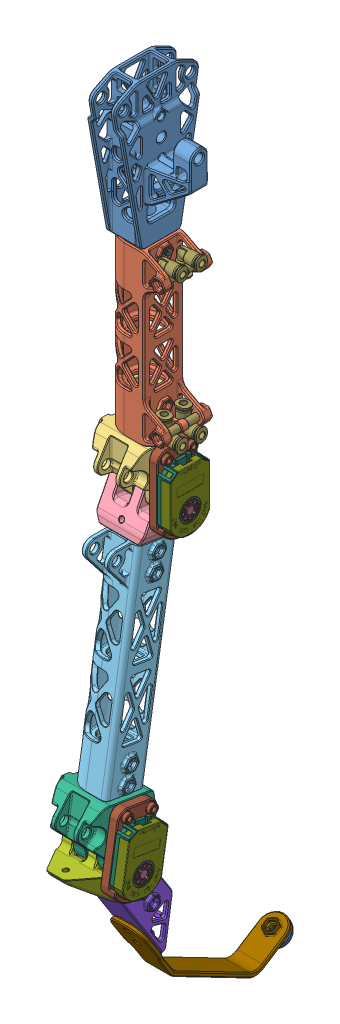
SolidWorks assembly AARL_Puppy_18_01_04_004, configuration Default. Lengths in mm.
Overall size (59.35 614.9 171.35).
42 component instances, 24 part files, 68 mates.
Components (placement in the parent):
- AARL_QR_FR_LE_PA_FR_028-2: AARL_QR_FR_LE_PA_FR_028 [Default] at (43.9453 155.049 100.762) size (52.49 127.48 60.54)
- AARL_QR_FR_LE_PL_BL_021-2: AARL_QR_FR_LE_PL_BL_021 [Default] at (43.9453 -3.9396 100.762) size (46.38 120.65 34.92)
- AARL_Puppy_18_01_04_037-1: AARL_Puppy_18_01_04_037 [Default] at (44.2247 -15.0521 100.762) x (0 0 1) z (1 0 0) size (54.18 69.85 37.51)
- AARL_QR_FR_LE_PL_BL_020-1: AARL_QR_FR_LE_PL_BL_020 [Default] at (44.1231 -40.4521 100.762) x (1 0 0) z (0 0.158913 0.987293) size (34.93 59.22 41.48)
- AARL_QR_FR_LE_PL_BL_024-1: AARL_QR_FR_LE_PL_BL_024 [Default] at (44.1231 -212.858 128.5122) x (1 0 0) z (0 0.158913 0.987293) size (30.96 149.23 44.46)
- AARL_Puppy_18_01_04_040-2: AARL_Puppy_18_01_04_040 [Default] at (95.2025 -223.8293 130.2781) x (0 -0.158913 -0.987293) z (-1 0 0) size (54.18 69.85 37.51)
- AARL_QR_FR_LE_PL_BL_013-1: AARL_QR_FR_LE_PL_BL_013 [Default] at (44.4025 -248.9066 134.3145) x (-1 0 0) z (0 0.539554 -0.841951) size (34.93 68.68 39.69)
- AARL_QR_FR_LE_PL_BL_014-1: AARL_QR_FR_LE_PL_BL_014 [Default] at (44.4025 -295.8585 104.2259) x (1 0 0) z (0 -0.539554 0.841951) size (27.78 53.98 25.4)
- AARL_QR_FR_LE_PL_BL_015-1: AARL_QR_FR_LE_PL_BL_015 [Default] at (44.4025 -304.904 115.3987) x (0 0.539554 -0.841951) z (1 0 0) size (70.12 107.32 25.4)
- AARL_QR_FR_LE_PL_BL_016-1: AARL_QR_FR_LE_PL_BL_016 [Default] at (44.4025 -363.4207 7.8107) x (0.981016 -0.104633 0.163276) z (0 0.841951 0.539554) size (18.99 18.99 9.09)
- AARL_Puppy_18_01_04_043-1: AARL_Puppy_18_01_04_043 [Default] at (61.7888 -40.4521 100.762) x (0 0 1) z (1 0 0) size (29.26 55.03 14.11)
- AARL_Puppy_18_01_04_043-2: AARL_Puppy_18_01_04_043 [Default] at (61.9666 -248.9066 134.3145) x (0 0.158913 0.987293) z (1 0 0) size (29.26 55.03 14.11)
- AARL_QR_PN_FT_002-QSML-4-4: AARL_QR_PN_FT_002-QSML-4 [Standard] at (65.4328 3.2604 107.6205) x (1 0 0) z (0 1 0) size (18.4 8 18.4)
- AARL_QR_PN_FT_002-QSML-4-6: AARL_QR_PN_FT_002-QSML-4 [Standard] at (65.4328 3.2604 93.9035) x (1 0 0) z (0 1 0) size (18.4 8 18.4)
- AARL_QR_PN_FT_002-QSML-4-7: AARL_QR_PN_FT_002-QSML-4 [Standard] at (65.4328 109.5104 93.9035) x (0 -1 0) z (1 0 0) size (18.4 8 18.4)
- AARL_QR_PN_FT_002-QSML-4-8: AARL_QR_PN_FT_002-QSML-4 [Standard] at (65.4328 109.5104 107.6205) x (0 -1 0) z (1 0 0) size (18.4 8 18.4)
- AARL_QR_HW_ST_002-8632T132_D_PROFILE_SHAFT_SHORT-3: AARL_QR_HW_ST_002-8632T132_D_PROFILE_SHAFT_SHORT [8632T132] at (51.9763 -40.4521 100.762) x (0 -0.999942 0.010793) z (-1 0 0) size (6.35 6.35 50.8)
- AARL_QR_HW_ST_002-8632T132_D_PROFILE_SHAFT_SHORT-4: AARL_QR_HW_ST_002-8632T132_D_PROFILE_SHAFT_SHORT [8632T132] at (52.1541 -248.9066 134.3145) x (0 0.841951 0.539554) z (-1 0 0) size (6.35 6.35 50.8)
- AARL_QR_HW_BE_004-6377K310_ULTRA-LOW-FRICTION DRY-RUNNING SLEEVE BEARING-1: AARL_QR_HW_BE_004-6377K310_ULTRA-LOW-FRICTION DRY-RUNNING SLEEVE BEARING [6377K31] at (58.6138 -40.4521 100.762) x (0 0.211282 -0.977425) z (1 0 0) size (9.55 9.55 6.35)
- AARL_QR_HW_BE_004-6377K310_ULTRA-LOW-FRICTION DRY-RUNNING SLEEVE BEARING-2: AARL_QR_HW_BE_004-6377K310_ULTRA-LOW-FRICTION DRY-RUNNING SLEEVE BEARING [6377K31] at (37.8747 -40.4521 100.762) x (0 0 -1) z (1 0 0) size (9.55 9.55 6.35)
- AARL_QR_EL_EN2-amt102-0048-i6350-s-1: AARL_QR_EL_EN2-amt102-0048-i6350-s [Default] at (71.9963 -40.4527 100.761) x (0 -0.000059 1) z (1 0 0) size (36.33 46.23 9.15)
  - AARL_QR_EL_EN2_001-CUI_DEVICES_amt-102-base-rev-k-1: AARL_QR_EL_EN2_001-CUI_DEVICES_amt-102-base-rev-k [Default] x (-1 0 0) z (0 0 -1) size (28.83 43.41 9.03)
  - AARL_QR_EL_EN2_002-CUI_DEVICES_amt-102-top-cover-rev-h-1: AARL_QR_EL_EN2_002-CUI_DEVICES_amt-102-top-cover-rev-h [Default] at (0 0 5.23) x (-1 0 0) z (0 0 -1) size (28.6 43.26 6.55)
  - AARL_QR_EL_EN2_003-CUI_DEVICES_amt-sleeve-rev-d(d)-1: AARL_QR_EL_EN2_003-CUI_DEVICES_amt-sleeve-rev-d(d) [Default] at (0 0 -2.42) x (0.999996 0.002864 0) z (0 0 1) size (10.79 10.79 7.8)
  - AARL_QR_EL_EN2_004-CUI_DEVICES_amt-hub-top-rev-d1-1: AARL_QR_EL_EN2_004-CUI_DEVICES_amt-hub-top-rev-d1 [Default] at (0 0 2.13) x (0.999996 0.002864 0) z (0 0 1) size (14 14 5.67)
  - AARL_QR_EL_EN2_005-CUI_DEVICES_amt-hub-bottom-rev-b-1: AARL_QR_EL_EN2_005-CUI_DEVICES_amt-hub-bottom-rev-b [Default] at (0 0 2.43) x (0.999998 -0.001942 0) z (0 0 1) size (17.3 17.3 3.2)
  - AARL_QR_EL_EN2_006-CUI_DEVICES_amt10x-shaft-adaptor-rev-e-1: AARL_QR_EL_EN2_006-CUI_DEVICES_amt10x-shaft-adaptor-rev-e [Default] at (0 0 0.03) x (0.999996 0.002864 0) z (0 0 1) size (11.8 11.8 7.8)
  - AARL_QR_EL_EN2_007-CUI_DEVICES_receiver-board-1: AARL_QR_EL_EN2_007-CUI_DEVICES_receiver-board [Default] at (72.2834 -20.351 3.03) x (-1 0 0) z (0 0 -1) size (26.5 26.62 0.41)
  - AARL_QR_EL_EN2_008-CUI_DEVICES_rotor-board-rev f-1: AARL_QR_EL_EN2_008-CUI_DEVICES_rotor-board-rev f [Default] at (0 0 2.13) x (0.807874 -0.589355 0) z (0 0 1) size (26 26 0.3)
  - AARL_QR_EL_EN2_009-CUI_DEVICES_transmitter-board amt10(amt-102)-1: AARL_QR_EL_EN2_009-CUI_DEVICES_transmitter-board amt10(amt-102) [Default] at (19.1596 -17.1102 1.22) x (-1 0 0) z (0 0 -1) size (26.63 38.43 4.41)
- AARL_QR_EL_EN2-amt102-0048-i6350-s-2: AARL_QR_EL_EN2-amt102-0048-i6350-s [Default] at (72.1741 -248.9073 134.3137) x (0 0.158855 0.987302) z (1 0 0) size (36.33 46.23 9.15)
  - AARL_QR_EL_EN2_001-CUI_DEVICES_amt-102-base-rev-k-1: AARL_QR_EL_EN2_001-CUI_DEVICES_amt-102-base-rev-k [Default] x (-1 0 0) z (0 0 -1) size (28.83 43.41 9.03)
  - AARL_QR_EL_EN2_002-CUI_DEVICES_amt-102-top-cover-rev-h-1: AARL_QR_EL_EN2_002-CUI_DEVICES_amt-102-top-cover-rev-h [Default] at (0 0 5.23) x (-1 0 0) z (0 0 -1) size (28.6 43.26 6.55)
  - AARL_QR_EL_EN2_003-CUI_DEVICES_amt-sleeve-rev-d(d)-1: AARL_QR_EL_EN2_003-CUI_DEVICES_amt-sleeve-rev-d(d) [Default] at (0 0 -2.42) x (0.999996 0.002864 0) z (0 0 1) size (10.79 10.79 7.8)
  - AARL_QR_EL_EN2_004-CUI_DEVICES_amt-hub-top-rev-d1-1: AARL_QR_EL_EN2_004-CUI_DEVICES_amt-hub-top-rev-d1 [Default] at (0 0 2.13) x (0.999996 0.002864 0) z (0 0 1) size (14 14 5.67)
  - AARL_QR_EL_EN2_005-CUI_DEVICES_amt-hub-bottom-rev-b-1: AARL_QR_EL_EN2_005-CUI_DEVICES_amt-hub-bottom-rev-b [Default] at (0 0 2.43) x (0.999998 -0.001942 0) z (0 0 1) size (17.3 17.3 3.2)
  - AARL_QR_EL_EN2_006-CUI_DEVICES_amt10x-shaft-adaptor-rev-e-1: AARL_QR_EL_EN2_006-CUI_DEVICES_amt10x-shaft-adaptor-rev-e [Default] at (0 0 0.03) x (0.999996 0.002864 0) z (0 0 1) size (11.8 11.8 7.8)
  - AARL_QR_EL_EN2_007-CUI_DEVICES_receiver-board-1: AARL_QR_EL_EN2_007-CUI_DEVICES_receiver-board [Default] at (72.2834 -20.351 3.03) x (-1 0 0) z (0 0 -1) size (26.5 26.62 0.41)
  - AARL_QR_EL_EN2_008-CUI_DEVICES_rotor-board-rev f-1: AARL_QR_EL_EN2_008-CUI_DEVICES_rotor-board-rev f [Default] at (0 0 2.13) x (0.807874 -0.589355 0) z (0 0 1) size (26 26 0.3)
  - AARL_QR_EL_EN2_009-CUI_DEVICES_transmitter-board amt10(amt-102)-1: AARL_QR_EL_EN2_009-CUI_DEVICES_transmitter-board amt10(amt-102) [Default] at (19.1596 -17.1102 1.22) x (-1 0 0) z (0 0 -1) size (26.63 38.43 4.41)
- AARL_QR_HW_CS_029-1: AARL_QR_HW_CS_029 [Default] at (26.813 110.3604 100.762) x (0 -0.235908 -0.971775) z (0 -0.971775 0.235908) size (4.65 34.79 4.65)
- AARL_QR_HW_CS_029-2: AARL_QR_HW_CS_029 [Default] at (26.813 97.6604 100.762) x (0 -0.235908 -0.971775) z (0 -0.971775 0.235908) size (4.65 34.79 4.65)
Mates (geometry in assembly coordinates):
- Concentric11: concentric aligned: cylinder of AARL_Puppy_18_01_04_040-2 through (75.6166 -248.9066 134.3145) axis (-1 0 0) radius 4.826; cylinder of AARL_QR_FR_LE_PL_BL_013-1 through (61.865 -248.9066 134.3145) axis (-1 0 0) radius 3.2385
- Coincident3: coincident anti-aligned: plane of AARL_Puppy_18_01_04_040-2; plane of AARL_QR_FR_LE_PL_BL_013-1 through (44.4025 -248.9066 134.3145) normal (-1 0 0)
- LimitAngle3: limit planar angle = 0.729498 rad anti-aligned: plane of AARL_QR_FR_LE_PL_BL_013-1 through (-20.4418 -252.7442 143.3393) normal (0 0.99672 -0.080932); plane of AARL_Puppy_18_01_04_040-2 through (100.8116 -231.1789 156.3642) normal (0 -0.689123 0.724644)
- Parallel4: parallel anti-aligned: plane of AARL_Puppy_18_01_04_040-2 through (100.8116 -210.5714 142.7184) normal (0 0.987293 -0.158913); plane of AARL_QR_FR_LE_PL_BL_013-1 through (44.4025 -294.5219 105.0824) normal (0 -0.841951 -0.539554)
- Parallel7: parallel anti-aligned: plane of AARL_QR_FR_LE_PL_BL_013-1 through (61.865 -248.7202 131.0814) normal (0 -0.539554 0.841951); plane of AARL_QR_HW_ST_002-8632T132_D_PROFILE_SHAFT_SHORT-4 through (26.7541 -248.7596 131.1429) normal (0 0.539554 -0.841951)
- Concentric25: concentric aligned: cylinder of AARL_Puppy_18_01_04_037-1 through (75.4388 -40.4521 100.762) axis (-1 0 0) radius 4.826; cylinder of AARL_QR_HW_BE_004-6377K310_ULTRA-LOW-FRICTION DRY-RUNNING SLEEVE BEARING-1 through (61.7888 -40.4521 100.762) axis (-1 0 0) radius 4.7752
- Coincident13: coincident anti-aligned: plane of AARL_Puppy_18_01_04_037-1 through (55.4388 -40.4521 100.762) normal (1 0 0); plane of AARL_QR_HW_BE_004-6377K310_ULTRA-LOW-FRICTION DRY-RUNNING SLEEVE BEARING-1 through (55.4388 -40.4521 100.762) normal (-1 0 0)
- Concentric26: concentric anti-aligned: cylinder of AARL_Puppy_18_01_04_037-1 through (21.0497 -40.4521 100.762) axis (1 0 0) radius 4.826; cylinder of AARL_QR_HW_BE_004-6377K310_ULTRA-LOW-FRICTION DRY-RUNNING SLEEVE BEARING-2 through (41.0497 -40.4521 100.762) axis (-1 0 0) radius 4.7752
- Coincident14: coincident anti-aligned: plane of AARL_Puppy_18_01_04_037-1 through (41.0497 -40.4521 100.762) normal (-1 0 0); plane of AARL_QR_HW_BE_004-6377K310_ULTRA-LOW-FRICTION DRY-RUNNING SLEEVE BEARING-2 through (41.0497 -40.4521 100.762) normal (1 0 0)
- Concentric27: concentric aligned: cylinder of AARL_Puppy_18_01_04_037-1 through (26.6606 -8.7021 91.872) axis (1 0 0) radius 1.5875; cylinder of AARL_Puppy_18_01_04_043-1 through (61.7888 -8.7021 91.872) axis (1 0 0) radius 1.5875
- Concentric28: concentric aligned: cylinder of AARL_Puppy_18_01_04_037-1 through (26.6606 -8.7021 109.652) axis (1 0 0) radius 1.5875; cylinder of AARL_Puppy_18_01_04_043-1 through (61.7888 -8.7021 109.652) axis (1 0 0) radius 1.5875
- Coincident15: coincident anti-aligned: plane of AARL_Puppy_18_01_04_037-1 through (61.7888 -40.4521 100.762) normal (1 0 0); plane of AARL_Puppy_18_01_04_043-1 through (61.7888 -40.2997 100.762) normal (-1 0 0)
- Concentric29: concentric aligned: cylinder of AARL_Puppy_18_01_04_040-2 through (26.8384 -218.9728 120.492) axis (1 0 0) radius 1.5875; cylinder of AARL_Puppy_18_01_04_043-2 through (61.9666 -218.9728 120.492) axis (1 0 0) radius 1.5875
- Concentric30: concentric aligned: cylinder of AARL_Puppy_18_01_04_040-2 through (26.8384 -216.1473 138.046) axis (1 0 0) radius 1.5875; cylinder of AARL_Puppy_18_01_04_043-2 through (61.9666 -216.1473 138.046) axis (1 0 0) radius 1.5875
- Coincident16: coincident anti-aligned: plane of AARL_Puppy_18_01_04_040-2 through (61.9666 -248.9066 134.3145) normal (1 0 0); plane of AARL_Puppy_18_01_04_043-2 through (61.9666 -248.7561 134.2903) normal (-1 0 0)
- Concentric31: concentric anti-aligned: cylinder of AARL_QR_EL_EN2-amt102-0048-i6350-s-1/AARL_QR_EL_EN2_001-CUI_DEVICES_amt-102-base-rev-k-1 through (68.2263 -24.7041 90.2845) axis (1 0 0) radius 1.9812; cylinder of AARL_Puppy_18_01_04_043-1 through (70.7663 -24.7041 90.2845) axis (-1 0 0) radius 1.8542
- Concentric32: concentric anti-aligned: cylinder of AARL_QR_EL_EN2-amt102-0048-i6350-s-1/AARL_QR_EL_EN2_001-CUI_DEVICES_amt-102-base-rev-k-1 through (68.2263 -49.4335 109.7407) axis (1 0 0) radius 1.9812; cylinder of AARL_Puppy_18_01_04_043-1 through (70.7663 -49.4337 109.7409) axis (-1 0 0) radius 1.8542
- Coincident17: coincident anti-aligned: plane of AARL_QR_EL_EN2-amt102-0048-i6350-s-1/AARL_QR_EL_EN2_001-CUI_DEVICES_amt-102-base-rev-k-1 through (68.2263 -30.0327 100.7616) normal (-1 0 0); plane of AARL_Puppy_18_01_04_043-1 through (68.2263 -40.2997 100.762) normal (1 0 0)
- Coincident18: coincident aligned: plane of AARL_QR_HW_ST_002-8632T132_D_PROFILE_SHAFT_SHORT-3 through (77.3763 -40.4521 100.762) normal (1 0 0); plane of AARL_QR_EL_EN2-amt102-0048-i6350-s-1/AARL_QR_EL_EN2_003-CUI_DEVICES_amt-sleeve-rev-d(d)-1 through (77.3763 -40.4527 100.761) normal (1 0 0)
- Concentric33: concentric anti-aligned: cylinder of AARL_QR_HW_ST_002-8632T132_D_PROFILE_SHAFT_SHORT-3 through (26.5763 -40.4521 100.762) axis (1 0 0) radius 3.175; cylinder of AARL_QR_HW_BE_004-6377K310_ULTRA-LOW-FRICTION DRY-RUNNING SLEEVE BEARING-2 through (41.0497 -40.4521 100.762) axis (-1 0 0) radius 3.2258
- Concentric34: concentric anti-aligned: cylinder of AARL_QR_EL_EN2-amt102-0048-i6350-s-2/AARL_QR_EL_EN2_001-CUI_DEVICES_amt-102-base-rev-k-1 through (68.4041 -235.0237 121.4676) axis (1 0 0) radius 1.9812; cylinder of AARL_Puppy_18_01_04_043-2 through (70.9441 -235.0237 121.4676) axis (-1 0 0) radius 1.8542
- Concentric35: concentric anti-aligned: cylinder of AARL_QR_EL_EN2-amt102-0048-i6350-s-2/AARL_QR_EL_EN2_001-CUI_DEVICES_amt-102-base-rev-k-1 through (68.4041 -256.347 144.6064) axis (1 0 0) radius 1.9812; cylinder of AARL_Puppy_18_01_04_043-2 through (70.9441 -256.3472 144.6066) axis (-1 0 0) radius 1.8542
- Coincident19: coincident anti-aligned: plane of AARL_QR_EL_EN2-amt102-0048-i6350-s-2/AARL_QR_EL_EN2_001-CUI_DEVICES_amt-102-base-rev-k-1 through (68.4041 -238.6196 132.6584) normal (-1 0 0); plane of AARL_Puppy_18_01_04_043-2 through (68.4041 -248.7561 134.2903) normal (1 0 0)
- Coincident20: coincident aligned: plane of AARL_QR_HW_ST_002-8632T132_D_PROFILE_SHAFT_SHORT-4 through (77.5541 -248.9066 134.3145) normal (1 0 0); plane of AARL_QR_EL_EN2-amt102-0048-i6350-s-2/AARL_QR_EL_EN2_003-CUI_DEVICES_amt-sleeve-rev-d(d)-1 through (77.5541 -248.9073 134.3137) normal (1 0 0)
- Concentric36: concentric aligned: cylinder of AARL_Puppy_18_01_04_040-2 through (21.2275 -248.9066 134.3145) axis (1 0 0) radius 4.826; cylinder of AARL_QR_HW_ST_002-8632T132_D_PROFILE_SHAFT_SHORT-4 through (26.7541 -248.9066 134.3145) axis (1 0 0) radius 3.175
- Parallel9: parallel anti-aligned: plane of AARL_QR_FR_LE_PL_BL_013-1 through (61.865 -248.7202 131.0814) normal (0 -0.539554 0.841951); plane of AARL_QR_HW_ST_002-8632T132_D_PROFILE_SHAFT_SHORT-4 through (26.7541 -248.7596 131.1429) normal (0 0.539554 -0.841951)
- Concentric37: concentric aligned: cylinder of AARL_QR_FR_LE_PL_BL_013-1 through (53.9275 -278.4828 115.3609) axis (1 0 0) radius 1.5875; cylinder of AARL_QR_FR_LE_PL_BL_014-1 through (31.7025 -278.4828 115.3609) axis (1 0 0) radius 1.5875
- Concentric38: concentric aligned: cylinder of AARL_QR_FR_LE_PL_BL_013-1 through (53.9275 -289.1756 108.5086) axis (1 0 0) radius 1.5875; cylinder of AARL_QR_FR_LE_PL_BL_014-1 through (31.7025 -289.1756 108.5086) axis (1 0 0) radius 1.5875
- Coincident21: coincident anti-aligned: plane of AARL_QR_FR_LE_PL_BL_013-1 through (53.9275 -289.3827 97.0628) normal (1 0 0); plane of AARL_QR_FR_LE_PL_BL_014-1 through (53.9275 -278.2756 126.8067) normal (-1 0 0)
- Concentric41: concentric anti-aligned: cylinder of AARL_QR_FR_LE_PL_BL_014-1 through (44.4025 -295.6886 89.2495) axis (0 -0.539554 0.841951) radius 1.5875; cylinder of AARL_QR_FR_LE_PL_BL_015-1 through (44.4025 -311.1069 113.3091) axis (0 0.539554 -0.841951) radius 1.5875
- Concentric42: concentric anti-aligned: cylinder of AARL_QR_FR_LE_PL_BL_014-1 through (44.4025 -306.3814 82.3972) axis (0 -0.539554 0.841951) radius 1.5875; cylinder of AARL_QR_FR_LE_PL_BL_015-1 through (44.4025 -321.7997 106.4568) axis (0 0.539554 -0.841951) radius 1.5875
- Coincident23: coincident anti-aligned: plane of AARL_QR_FR_LE_PL_BL_014-1 through (57.1025 -301.3743 115.7752) normal (0 -0.539554 0.841951); plane of AARL_QR_FR_LE_PL_BL_015-1 through (53.9275 -304.0475 114.0621) normal (0 0.539554 -0.841951)
- Concentric43: concentric aligned: cylinder of AARL_QR_FR_LE_PL_BL_015-1 through (44.4025 -363.4207 7.8107) axis (0 0.841951 0.539554) radius 1.5875; cylinder of AARL_QR_FR_LE_PL_BL_016-1 through (44.4025 -363.4207 7.8107) axis (0 0.841951 0.539554) radius 1.5875
- Coincident24: coincident anti-aligned: plane of AARL_QR_FR_LE_PL_BL_015-1 through (53.9275 -377.7233 30.1293) normal (0 -0.841951 -0.539554); plane of AARL_QR_FR_LE_PL_BL_016-1 through (45.9599 -363.5868 8.0699) normal (0 0.841951 0.539554)
- Concentric47: concentric: cylinder of AARL_QR_FR_LE_PL_BL_019-2 through (29.65 -45.2146 100.762) axis (1 0 0) radius 1.5875; cylinder of AARL_Puppy_18_01_04_037-1 through (26.6606 -45.2146 100.762) axis (1 0 0) radius 1.5875
- Concentric48: concentric: cylinder of AARL_QR_FR_LE_PL_BL_019-2 through (29.65 -57.9146 100.762) axis (1 0 0) radius 1.5875; cylinder of AARL_Puppy_18_01_04_037-1 through (26.6606 -57.9146 100.762) axis (1 0 0) radius 1.5875
- Coincident26: coincident: plane of AARL_QR_FR_LE_PL_BL_019-2 through (55.0578 -38.8646 89.6495) normal (-1 0 0); plane of AARL_Puppy_18_01_04_037-1 through (55.0578 -38.8646 111.5951) normal (1 0 0)
- Concentric50: concentric anti-aligned: cylinder of AARL_QR_FR_LE_PL_BL_020-1 through (61.5856 -40.4521 100.762) axis (-1 0 0) radius 3.2385; cylinder of AARL_QR_HW_ST_002-8632T132_D_PROFILE_SHAFT_SHORT-3 through (26.5763 -40.4521 100.762) axis (1 0 0) radius 3.175
- Width4: width anti-aligned: plane of AARL_QR_FR_LE_PL_BL_020-1 through (34.3822 -38.0213 90.7336) normal (1 0 0); plane of AARL_QR_FR_LE_PL_BL_020-1 through (44.5422 -38.0213 90.7336) normal (-1 0 0); plane of AARL_Puppy_18_01_04_037-1 through (44.2247 -21.4021 121.5011) normal (1 0 0); plane of AARL_Puppy_18_01_04_037-1 through (34.6997 -40.4521 100.762) normal (-1 0 0)
- Parallel10: parallel: plane of AARL_QR_FR_LE_PL_BL_019-2 through (43.9453 56.3874 115.0495) normal (0 0 1); plane of AARL_QR_FR_LE_PL_BL_020-1
- Concentric51: concentric: cylinder of AARL_QR_FR_LE_PL_BL_019-2 through (70.9328 -51.5646 111.8745) axis (0 0 1) radius 1.5875; cylinder of AARL_QR_PN_FT_002-QSML-4-4 through (70.9328 -51.5646 103.6205) axis (0 0 -1) radius 1.6
- Width5: width: plane of AARL_QR_PN_FT_002-QSML-4-4 through (70.9328 8.7604 111.6205) normal (0 0 1); plane of AARL_QR_PN_FT_002-QSML-4-4 through (70.9328 8.7604 103.6205) normal (0 0 -1); plane of AARL_QR_FR_LE_PL_BL_019-2 through (43.9453 -3.9396 111.8745) normal (0 0 -1); plane of AARL_QR_FR_LE_PL_BL_019-2 through (43.9453 -3.9396 103.3665) normal (0 0 1)
- Concentric55: concentric aligned: cylinder of AARL_QR_FR_LE_PA_FR_028-2 through (31.2453 110.3604 100.762) axis (1 0 0) radius 1.5875; cylinder of AARL_QR_FR_LE_PL_BL_021-2 through (29.6578 110.3604 100.762) axis (1 0 0) radius 1.5875
- Concentric56: concentric aligned: cylinder of AARL_QR_FR_LE_PA_FR_028-2 through (31.2453 97.6604 100.762) axis (1 0 0) radius 1.5875; cylinder of AARL_QR_FR_LE_PL_BL_021-2 through (29.6578 97.6604 100.762) axis (1 0 0) radius 1.5875
- Coincident29: coincident anti-aligned: plane of AARL_QR_FR_LE_PA_FR_028-2 through (55.0578 59.8795 89.6495) normal (1 0 0); plane of AARL_QR_FR_LE_PL_BL_021-2 through (55.0578 116.7104 111.8745) normal (-1 0 0)
- Concentric58: concentric anti-aligned: cylinder of AARL_QR_FR_LE_PL_BL_021-2 through (70.9328 8.7604 111.8745) axis (0 0 1) radius 1.5875; cylinder of AARL_QR_PN_FT_002-QSML-4-4 through (70.9328 8.7604 103.6205) axis (0 0 -1) radius 1.6
- Width7: width anti-aligned: plane of AARL_QR_PN_FT_002-QSML-4-4 through (70.9328 8.7604 111.6205) normal (0 0 1); plane of AARL_QR_PN_FT_002-QSML-4-4 through (70.9328 8.7604 103.6205) normal (0 0 -1); plane of AARL_QR_FR_LE_PL_BL_021-2 through (43.9453 -3.9396 111.8745) normal (0 0 -1); plane of AARL_QR_FR_LE_PL_BL_021-2 through (43.9453 -3.9396 103.3665) normal (0 0 1)
- Concentric59: concentric aligned: cylinder of AARL_QR_FR_LE_PL_BL_021-2 through (70.9328 8.7604 89.6495) axis (0 0 -1) radius 1.5875; cylinder of AARL_QR_PN_FT_002-QSML-4-6 through (70.9328 8.7604 89.9035) axis (0 0 -1) radius 1.6
- Width8: width aligned: plane of AARL_QR_PN_FT_002-QSML-4-6 through (70.9328 8.7604 97.9035) normal (0 0 1); plane of AARL_QR_PN_FT_002-QSML-4-6 through (70.9328 8.7604 89.9035) normal (0 0 -1); plane of AARL_QR_FR_LE_PL_BL_021-2 through (43.9453 -3.9396 89.6495) normal (0 0 1); plane of AARL_QR_FR_LE_PL_BL_021-2 through (43.9453 -3.9396 98.1575) normal (0 0 -1)
- Concentric60: concentric aligned: cylinder of AARL_QR_FR_LE_PL_BL_021-2 through (70.9328 104.0104 89.6495) axis (0 0 -1) radius 1.5875; cylinder of AARL_QR_PN_FT_002-QSML-4-7 through (70.9328 104.0104 89.9035) axis (0 0 -1) radius 1.6
- Width9: width anti-aligned: plane of AARL_QR_PN_FT_002-QSML-4-7 through (70.9328 104.0104 97.9035) normal (0 0 1); plane of AARL_QR_PN_FT_002-QSML-4-7 through (70.9328 104.0104 89.9035) normal (0 0 -1); plane of AARL_QR_FR_LE_PL_BL_021-2 through (43.9453 -3.9396 98.1575) normal (0 0 -1); plane of AARL_QR_FR_LE_PL_BL_021-2 through (43.9453 -3.9396 89.6495) normal (0 0 1)
- Concentric61: concentric anti-aligned: cylinder of AARL_QR_FR_LE_PL_BL_021-2 through (70.9328 104.0104 111.8745) axis (0 0 1) radius 1.5875; cylinder of AARL_QR_PN_FT_002-QSML-4-8 through (70.9328 104.0104 103.6205) axis (0 0 -1) radius 1.6
- Width10: width anti-aligned: plane of AARL_QR_PN_FT_002-QSML-4-8 through (70.9328 104.0104 111.6205) normal (0 0 1); plane of AARL_QR_PN_FT_002-QSML-4-8 through (70.9328 104.0104 103.6205) normal (0 0 -1); plane of AARL_QR_FR_LE_PL_BL_021-2 through (43.9453 -3.9396 111.8745) normal (0 0 -1); plane of AARL_QR_FR_LE_PL_BL_021-2 through (43.9453 -3.9396 103.3665) normal (0 0 1)
- Concentric62: concentric anti-aligned: cylinder of AARL_QR_PN_FT_002-QSML-4-6 through (65.4328 16.7604 93.9035) axis (0 -1 0) radius 2; cylinder of AARL_QR_PN_FT_002-QSML-4-7 through (65.4328 96.0104 93.9035) axis (0 1 0) radius 2
- Concentric63: concentric anti-aligned: cylinder of AARL_QR_PN_FT_002-QSML-4-4 through (65.4328 16.7604 107.6205) axis (0 -1 0) radius 2; cylinder of AARL_QR_PN_FT_002-QSML-4-8 through (65.4328 96.0104 107.6205) axis (0 1 0) radius 2
- Concentric64: concentric aligned: cylinder of AARL_QR_FR_LE_PL_BL_021-2 through (29.6578 15.1104 100.762) axis (1 0 0) radius 1.5875; cylinder of AARL_Puppy_18_01_04_037-1 through (26.6606 15.1104 100.762) axis (1 0 0) radius 1.5875
- Concentric65: concentric aligned: cylinder of AARL_QR_FR_LE_PL_BL_021-2 through (29.6578 2.4104 100.762) axis (1 0 0) radius 1.5875; cylinder of AARL_Puppy_18_01_04_037-1 through (26.6606 2.4104 100.762) axis (1 0 0) radius 1.5875
- Coincident30: coincident anti-aligned: plane of AARL_QR_FR_LE_PL_BL_021-2 through (55.0578 21.4604 89.6495) normal (-1 0 0); plane of AARL_Puppy_18_01_04_037-1 through (55.0578 21.4604 111.5951) normal (1 0 0)
- Concentric72: concentric aligned: cylinder of AARL_QR_FR_LE_PL_BL_020-1 through (26.6606 -71.7986 105.8075) axis (1 0 0) radius 1.5875; cylinder of AARL_QR_FR_LE_PL_BL_024-1 through (29.8356 -71.7986 105.8075) axis (1 0 0) radius 1.5875
- Concentric73: concentric aligned: cylinder of AARL_QR_FR_LE_PL_BL_020-1 through (26.6606 -84.3372 107.8256) axis (1 0 0) radius 1.5875; cylinder of AARL_QR_FR_LE_PL_BL_024-1 through (29.8356 -84.3372 107.8256) axis (1 0 0) radius 1.5875
- Coincident33: coincident anti-aligned: plane of AARL_QR_FR_LE_PL_BL_020-1 through (55.2356 -88.8406 119.806) normal (1 0 0); plane of AARL_QR_FR_LE_PL_BL_024-1 through (55.2356 -63.7634 115.7696) normal (-1 0 0)
- Concentric74: concentric aligned: cylinder of AARL_QR_FR_LE_PL_BL_024-1 through (29.8356 -194.0501 125.4849) axis (1 0 0) radius 1.5875; cylinder of AARL_Puppy_18_01_04_040-2 through (26.8384 -194.0501 125.4849) axis (1 0 0) radius 1.5875
- Concentric75: concentric aligned: cylinder of AARL_QR_FR_LE_PL_BL_024-1 through (29.8356 -206.5887 127.5031) axis (1 0 0) radius 1.5875; cylinder of AARL_Puppy_18_01_04_040-2 through (26.8384 -206.5887 127.5031) axis (1 0 0) radius 1.5875
- Coincident34: coincident anti-aligned: plane of AARL_QR_FR_LE_PL_BL_024-1 through (55.2356 -189.5467 113.5045) normal (-1 0 0); plane of AARL_Puppy_18_01_04_040-2 through (55.2356 -189.5023 113.7803) normal (1 0 0)
- Concentric76: concentric anti-aligned: cylinder of AARL_QR_FR_LE_PL_BL_021-2 through (29.6578 110.3604 100.762) axis (1 0 0) radius 1.5875; cylinder of AARL_QR_HW_CS_029-1 through (26.813 110.3604 100.762) axis (-1 0 0) radius 1.4224
- Tangent1: tangent anti-aligned: cylinder of AARL_QR_FR_LE_PL_BL_021-2 through (43.9453 21.4604 100.762) axis (0 -1 0) radius 14.2875; plane of AARL_QR_HW_CS_029-1 through (29.6578 110.0249 99.3797) normal (1 0 0)
- Concentric77: concentric anti-aligned: cylinder of AARL_QR_FR_LE_PL_BL_021-2 through (29.6578 97.6604 100.762) axis (1 0 0) radius 1.5875; cylinder of AARL_QR_HW_CS_029-2 through (26.813 97.6604 100.762) axis (-1 0 0) radius 1.4224
- Tangent2: tangent anti-aligned: cylinder of AARL_QR_FR_LE_PL_BL_021-2 through (43.9453 21.4604 100.762) axis (0 -1 0) radius 14.2875; plane of AARL_QR_HW_CS_029-2 through (29.6578 97.3249 99.3797) normal (1 0 0)
